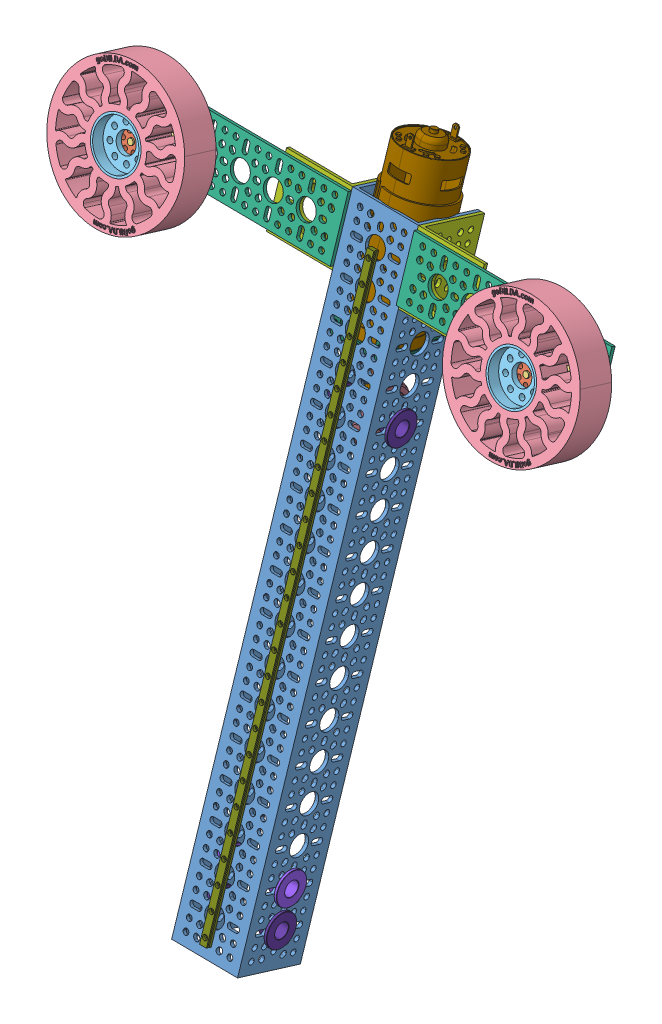
SolidWorks assembly 总装, configuration 默认. Lengths in mm.
Overall size (409.26 477.79 195.31).
38 component instances, 17 part files, 32 mates.
Components (placement in the parent):
- 432mm-U型梁-1: 432mm-U型梁 [默认] at (-52.5612 -100.8788 473.6792) x (0.999953 -0.009656 0) z (0.002854 0.295554 0.955322) size (48 432 48)
- 发射法兰1-2: 发射法兰1 [默认] at (95.3037 298.6557 389.1988) x (0.597612 -0.766469 0.235342) z (0.801781 0.57024 -0.178814) size (30 11 30)
- 发射无刷电机-2: 发射无刷电机 [默认] at (95.2101 288.9616 357.8642) x (-0.009225 -0.955277 0.295568) z (-0.999953 0.009656 0) size (58.5 35.4 58.5)
- 摩擦轮-2: 摩擦轮 [默认] at (94.6021 282.6082 387.0905) x (-0.954993 -0.28256 0.09027) z (-0.002854 -0.295554 -0.955322) size (96 96 24)
  - 摩擦轮.STEP-1: 摩擦轮.STEP [默认] at origin size (96 96 24)
    - 3613-0014-0096 Rubber.STEP-1: 3613-0014-0096 Rubber.STEP [默认] at (-5.0141 13.8433 -6.759) size (96 96 24)
    - 3613-0014-0096 Core.STEP-1: 3613-0014-0096 Core.STEP [默认] at (-5.0141 13.8433 -6.759) x (1 0 0) z (0 -1 0) size (35.2 24 35.2)
- 5孔平板-2: 5孔平板 [默认] at (119.072 274.5458 384.7583) x (0.002854 0.295554 0.955322) z (-0.009225 -0.955277 0.295568) size (2.5 144 43)
- 48x48-L形支架-2: 48x48-L形支架 [默认] at (-22.5815 259.3374 339.6418) x (0.002854 0.295554 0.955322) z (-0.999953 0.009656 0) size (48 48 48)
- 装配体3-2: 装配体3 [默认] at (-128.0634 200.7559 231.0431) x (0.002854 0.295554 0.955322) z (0.999953 -0.009656 0) size (95.3 120.73 180.37)
  - 发射法兰1-1: 发射法兰1 [默认] at (180.6617 -48.8364 -65.5887) x (0 1 0) z (0 0 1) size (30 11 30)
  - 发射无刷电机-1: 发射无刷电机 [默认] at (147.8617 -48.8364 -65.5887) x (0 -1 0) z (0 0 1) size (58.5 35.4 58.5)
  - 摩擦轮-1: 摩擦轮 [默认] at (173.9027 -63.5495 -65.0421) x (0 -0.305413 0.95222) z (-1 0 0) size (96 96 24)
    - 摩擦轮.STEP-1: 摩擦轮.STEP [默认] at origin size (96 96 24)
      - 3613-0014-0096 Rubber.STEP-1: 3613-0014-0096 Rubber.STEP [默认] at (-5.0141 13.8433 -6.759) size (96 96 24)
      - 3613-0014-0096 Core.STEP-1: 3613-0014-0096 Core.STEP [默认] at (-5.0141 13.8433 -6.759) x (1 0 0) z (0 -1 0) size (35.2 24 35.2)
  - 5孔平板-1: 5孔平板 [默认] at (169.3617 -70.3364 -89.5887) x (1 0 0) z (0 -1 0) size (2.5 144 43)
  - 48x48-L形支架-1: 48x48-L形支架 [默认] at (121.3617 -72.8364 51.9113) size (48 48 48)
- 2306-4008-0014 assembly-1: 2306-4008-0014 assembly [默认] at (-186.8079 96.5973 629.512) x (0 0.597801 0.801645) z (-0.223733 -0.781323 0.582647)
- 花篮螺丝-1: 花篮螺丝 [默认] at (-71.9313 -35.5534 412.0649) x (0.008275 0.856874 0.51546) z (0.999953 -0.009656 0)
- 铜套1-5: 铜套1 [默认] at (-78.1786 -61.1289 438.9525) x (0.999953 -0.009656 0) z (0 0 1) size (10 22 22)
- 铜套1-6: 铜套1 [默认] at (-26.181 -61.631 438.9525) x (-0.999953 0.009656 0) z (0 0 1) size (10 22 22)
- 皮带电机装配体-3: 皮带电机装配体 [默认] at (17.3534 305.199 468.5412) x (0.009225 0.955277 -0.295568) z (0.002854 0.295554 0.955322) size (182.3 67.11 64.42)
  - 发射轮电机1-1: 发射轮电机1 [默认] at (-31.948 68.6302 -206.7966) size (148.5 67.11 64.42)
  - 3204-0002-0002 assembly-1: 3204-0002-0002 assembly [默认] at (-82.9257 129.4143 -179.1986) x (0 1 0) z (0 0 1) size (28.67 52.38 42.6)
    - 2306-4008-0014 assembly(2)-1: 2306-4008-0014 assembly(2) [默认] at (-86.5036 -22.1715 14.0673) x (0 1 0) z (-0.223733 0 0.97465) size (15.4 23.81 24.42)
      - 2306-4008-0014-1: 2306-4008-0014 [默认] at (-4.2928 -28.4802 22.5212) size (15.32 23.81 24.42)
      - 2306-4008-0014 clamp-1: 2306-4008-0014 clamp [默认] at (-4.2932 -28.4802 22.5212) size (9.55 8.86 18.72)
      - 2800-0004-0012_90128A207-1: 2800-0004-0012_90128A207 [默认] at (-8.9015 -37.2302 16.6212) x (0.549526 0 0.835476) z (0 -1 0) size (7 7 16.17)
      - 2800-0004-0012_90128A207-2: 2800-0004-0012_90128A207 [默认] at (-8.9015 -37.2302 28.4212) x (0.549526 0 -0.835476) z (0 -1 0) size (7 7 16.17)
    - 2307-0014-0028-1: 2307-0014-0028 [默认] at (-76.6728 -4.8452 42.3896) size (6.41 42.6 42.6)
  - 齿轮组法兰-1: 齿轮组法兰 [默认] at (-78.0805 56.1302 -136.809) x (0 1 0) z (0 0 1) size (12 30 30) (hidden)
  - 电机转向座1-1: 电机转向座1 [默认] at (-41.0801 65.9902 -136.809) x (0 0 -1) z (0 -1 0) size (43.24 12.23 43.24)
- 滑轨9-1: 滑轨9 [默认] at (-54.9831 -92.7733 473.7957) x (0.999953 -0.009656 0) z (-0.009225 -0.955277 0.295568) size (73.65 3.7 429.69)
- 铜套-2: 铜套 [默认] at (-75.7432 191.0643 360.9227) x (0.999953 -0.009656 0) z (0 0 1) size (10 22 22)
- 铜套-3: 铜套 [默认] at (-23.7457 190.5622 360.9227) x (-0.999953 0.009656 0) z (-0.009078 -0.94012 -0.340724) size (10 22 22)
- 铜套-4: 铜套 [默认] at (-78.4 -84.0555 446.0461) x (0.999953 -0.009656 0) z (0.000026 0.002689 0.999996) size (10 22 22)
- 铜套-5: 铜套 [默认] at (-26.4024 -84.5576 446.0461) x (-0.999953 0.009656 0) z (-0.009078 -0.94012 -0.340724) size (10 22 22)
Mates (geometry in assembly coordinates):
- 重合22: coincident aligned: circle of 432mm-U型梁-1; circle of 装配体3-2/48x48-L形支架-1
- 平行4: parallel aligned: plane of 432mm-U型梁-1 through (-24.5701 312.3081 348.3823) normal (0.002854 0.295554 0.955322); plane of 装配体3-2/5孔平板-1 through (-72.5838 311.1223 351.5095) normal (0.002854 0.295554 0.955322)
- 同心82: concentric anti-aligned: circle of 432mm-U型梁-1; circle of 铜套1-5
- 重合97: coincident anti-aligned: plane of 432mm-U型梁-1 through (-72.7048 298.585 302.5268) normal (-0.999953 0.009656 0); plane of 铜套1-5 through (-76.1787 -61.1482 438.9525) normal (0.999953 -0.009656 0)
- 同心83: concentric aligned: circle of 432mm-U型梁-1; circle of 铜套1-6
- 重合100: coincident anti-aligned: plane of 432mm-U型梁-1 through (-24.7071 298.1215 302.5268) normal (0.999953 -0.009656 0); plane of 铜套1-6 through (-28.1809 -61.6117 438.9525) normal (-0.999953 0.009656 0)
- 同心5: concentric anti-aligned: circle of 发射法兰1-2; circle of 发射无刷电机-2
- 重合158: coincident anti-aligned: circle of 发射法兰1-2; plane of 发射无刷电机-2 through (95.377 306.2531 381.6143) normal (0.002854 0.295554 0.955322)
- 同心6: concentric anti-aligned: circle of 发射法兰1-2; circle of 摩擦轮-2/摩擦轮.STEP-1/3613-0014-0096 Core.STEP-1
- 重合5: coincident anti-aligned: plane of 发射法兰1-2 through (95.3037 298.6557 389.1988) normal (0.002854 0.295554 0.955322); plane of 摩擦轮-2/摩擦轮.STEP-1/3613-0014-0096 Core.STEP-1 through (95.3037 298.6557 389.1988) normal (-0.002854 -0.295554 -0.955322)
- 同心2: concentric anti-aligned: circle of 发射无刷电机-2; circle of 5孔平板-2
- 重合3: coincident anti-aligned: plane of 发射无刷电机-2 through (95.2101 288.9616 357.8642) normal (-0.002854 -0.295554 -0.955322); plane of 5孔平板-2 through (-24.9827 269.5819 364.2189) normal (0.002854 0.295554 0.955322)
- 同心1: concentric aligned: circle of 5孔平板-2; circle of 48x48-L形支架-2
- 平行1: parallel aligned: plane of 5孔平板-2 through (119.072 274.5458 384.7583) normal (0.999953 -0.009656 0); plane of 48x48-L形支架-2 through (23.4205 311.1057 345.994) normal (0.999953 -0.009656 0)
- 同心129: concentric anti-aligned: circle of 432mm-U型梁-1; circle of 48x48-L形支架-2
- 重合159: coincident aligned: plane of 432mm-U型梁-1 through (-27.207 298.1457 302.5268) normal (-0.002854 -0.295554 -0.955322); plane of 48x48-L形支架-2 through (23.2907 297.658 302.5268) normal (-0.002854 -0.295554 -0.955322)
- 重合160: coincident anti-aligned: plane of 432mm-U型梁-1 through (-24.7071 298.1215 302.5268) normal (0.999953 -0.009656 0); plane of 48x48-L形支架-2 through (-24.5701 312.3081 348.3823) normal (-0.999953 0.009656 0)
- 同心135: concentric anti-aligned: circle of 432mm-U型梁-1; circle of 皮带电机装配体-3/3204-0002-0002 assembly-1/2307-0014-0028-1
- 重合171: coincident anti-aligned: plane of 432mm-U型梁-1 through (-27.0771 311.5934 345.994) normal (-0.999953 0.009656 0); plane of 皮带电机装配体-3/电机转向座1-1 through (-27.9889 217.1701 352.7035) normal (0.999953 -0.009656 0)
- 平行13: parallel aligned: plane of 432mm-U型梁-1 through (-27.207 298.1457 302.5268) normal (-0.002854 -0.295554 -0.955322); plane of 皮带电机装配体-3/电机转向座1-1 through (-49.4276 223.6256 328.2649) normal (-0.002854 -0.295554 -0.955322)
- 同心138: concentric anti-aligned: circle of 432mm-U型梁-1; circle of 滑轨9-1
- 同心139: concentric anti-aligned: circle of 432mm-U型梁-1; circle of 滑轨9-1
- 重合176: coincident anti-aligned: plane of 432mm-U型梁-1 through (-24.5701 312.3081 348.3823) normal (0.002854 0.295554 0.955322); plane of 滑轨9-1 through (-46.2934 289.2894 355.5686) normal (-0.002854 -0.295554 -0.955322)
- Concentric1: concentric aligned: cylinder of 432mm-U型梁-1 through (-63.7438 190.9485 360.9227) axis (-0.999953 0.009656 0) radius 7; cylinder of 铜套-2 through (-65.7437 190.9678 360.9227) axis (-0.999953 0.009656 0) radius 7
- Coincident2: coincident anti-aligned: plane of 432mm-U型梁-1 through (-72.7048 298.585 302.5268) normal (-0.999953 0.009656 0); plane of 铜套-2 through (-73.7433 191.045 360.9227) normal (0.999953 -0.009656 0)
- Concentric2: concentric aligned: cylinder of 432mm-U型梁-1 through (-35.7451 190.6781 360.9227) axis (0.999953 -0.009656 0) radius 7; cylinder of 铜套-3 through (-33.7452 190.6588 360.9227) axis (0.999953 -0.009656 0) radius 7
- Coincident3: coincident anti-aligned: plane of 432mm-U型梁-1 through (-24.7071 298.1215 302.5268) normal (0.999953 -0.009656 0); plane of 铜套-3 through (-25.7456 190.5815 360.9227) normal (-0.999953 0.009656 0)
- Concentric3: concentric aligned: cylinder of 432mm-U型梁-1 through (-66.4005 -84.1714 446.0461) axis (-0.999953 0.009656 0) radius 7; cylinder of 铜套-4 through (-68.4005 -84.1521 446.0461) axis (-0.999953 0.009656 0) radius 7
- Coincident4: coincident anti-aligned: plane of 432mm-U型梁-1 through (-72.7048 298.585 302.5268) normal (-0.999953 0.009656 0); plane of 铜套-4 through (-76.4001 -84.0748 446.0461) normal (0.999953 -0.009656 0)
- Concentric4: concentric aligned: cylinder of 432mm-U型梁-1 through (-38.4019 -84.4418 446.0461) axis (0.999953 -0.009656 0) radius 7; cylinder of 铜套-5 through (-36.4019 -84.4611 446.0461) axis (0.999953 -0.009656 0) radius 7
- Coincident5: coincident anti-aligned: plane of 432mm-U型梁-1 through (-24.7071 298.1215 302.5268) normal (0.999953 -0.009656 0); plane of 铜套-5 through (-28.4023 -84.5383 446.0461) normal (-0.999953 0.009656 0)
- Coincident9: coincident anti-aligned: plane of 5孔平板-2 through (-24.5701 312.3081 348.3823) normal (-0.002854 -0.295554 -0.955322); plane of 48x48-L形支架-2 through (23.4277 311.8446 348.3823) normal (0.002854 0.295554 0.955322)
